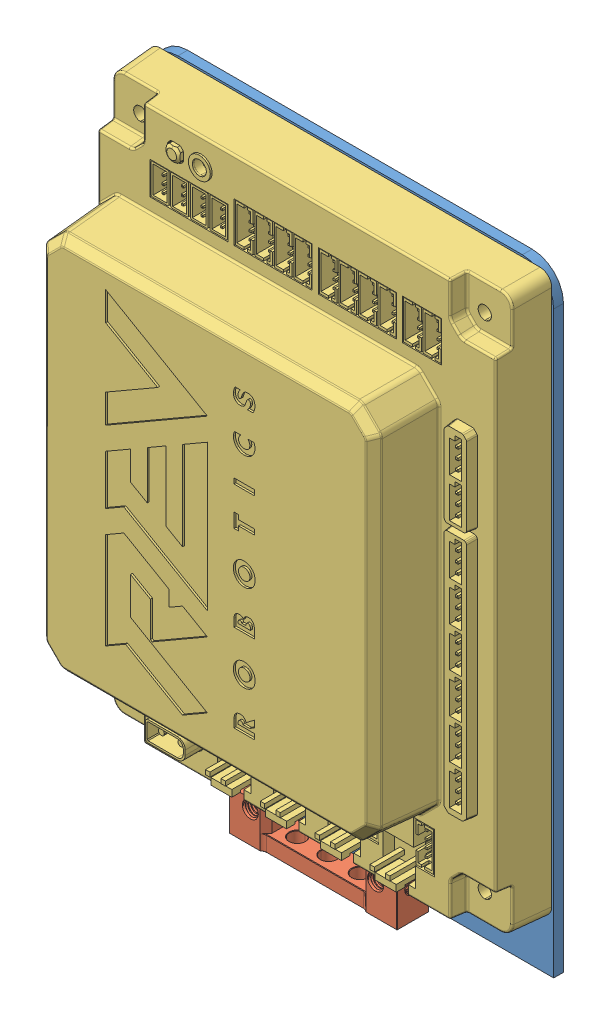
SolidWorks assembly Rev Hubs Assembly, configuration Default. Lengths in mm.
Overall size (104 156 32.08).
3 component instances, 3 part files, 6 mates.
Components (placement in the parent):
- Rev hub mounting plate leauge champs-1: Rev hub mounting plate leauge champs [Default] at (61.2961 36.546 148.6052) size (104 156 2.5)
- dual block.step-1: dual block.step [Default] at (61.2961 20.546 172.6052) x (0 0 1) z (0 -1 0) size (9.5 43 12)
- REV-31-1595.step-1: REV-31-1595.step [Default] at (61.2961 100.546 151.0341) x (1 0 0) z (0 -1 0) size (103 29.58 143)
Mates (geometry in assembly coordinates):
- Coincident1: coincident: plane of Rev hub mounting plate leauge champs-1 through (61.2961 36.546 151.1052) normal (0 0 1); plane of dual block.step-1 through (39.7961 20.546 151.1052) normal (0 0 -1)
- Concentric2: concentric anti-aligned: cylinder of Rev hub mounting plate leauge champs-1 through (77.2961 24.546 151.1052) axis (0 0 -1) radius 2; circle of dual block.step-1
- Coincident3: coincident aligned: plane of Rev hub mounting plate leauge champs-1 through (113.2961 16.546 151.1052) normal (0 -1 0); plane of dual block.step-1 through (61.2961 16.546 173.8552) normal (0 -1 0)
- Concentric3: concentric aligned: cylinder of Rev hub mounting plate leauge champs-1 through (17.2961 36.546 151.1052) axis (0 0 -1) radius 2; cylinder of REV-31-1595.step-1 through (17.2961 36.546 164.7052) axis (0 0 -1) radius 1.7
- Concentric5: concentric anti-aligned: circle of Rev hub mounting plate leauge champs-1; cylinder of REV-31-1595.step-1 through (105.2961 36.546 164.7052) axis (0 0 -1) radius 1.7
- Coincident4: coincident anti-aligned: plane of Rev hub mounting plate leauge champs-1 through (61.2961 36.546 151.1052) normal (0 0 1); plane of REV-31-1595.step-1 through (61.2961 100.546 151.1052) normal (0 0 -1)
